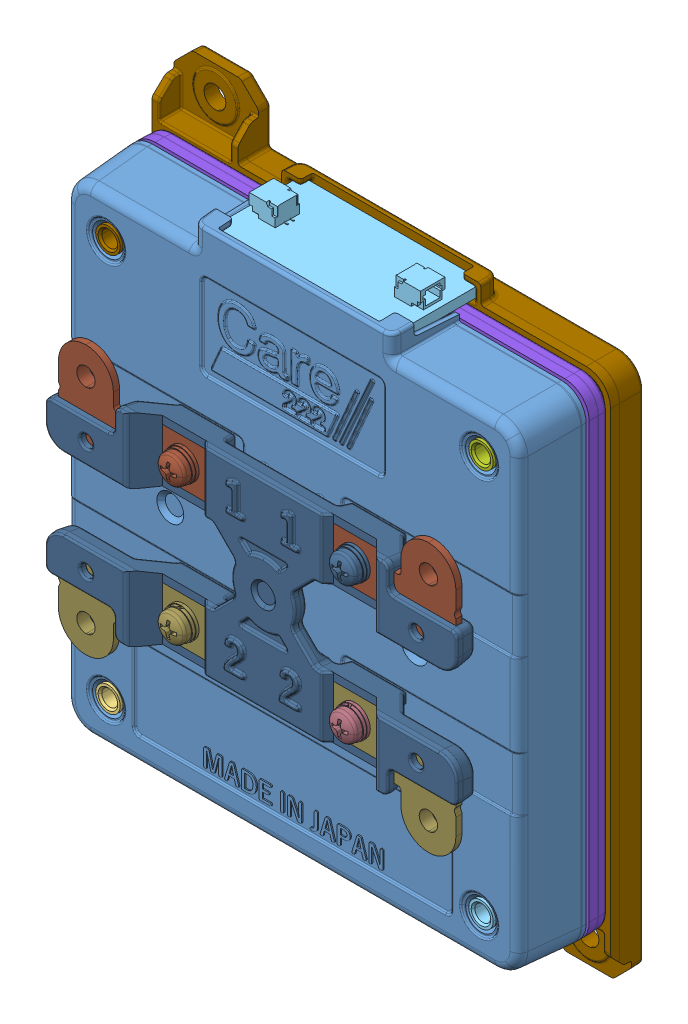
SolidWorks assembly emitter, configuration Default. Lengths in mm.
Overall size (75 97 26.91).
35 component instances, 31 part files, 0 mates.
Components (placement in the parent):
- emitter.step-1: emitter.step [Default] at origin size (75 97 26.91)
  - DRW1103739_UXFL70-222B4-UIA-Z1.STEP.step-1: DRW1103739_UXFL70-222B4-UIA-Z1.STEP.step [Default] at (-18.8418 87.9656 71.8261) size (75 97 26.91)
    - Z01_DRW1103184_LampCaseA.STEP.step-1: Z01_DRW1103184_LampCaseA.STEP.step [Default] at (0 3.0667 9.49) x (1 0 0) z (0 -1 0) size (75 10.8 82.07)
      - Z01_DRW1103184_LampCaseA-Part-1.STEP.step-1: Z01_DRW1103184_LampCaseA-Part-1.STEP.step [Default] at origin size (75 10.8 82.07)
      - Z01_DRW1103184_LampCaseA-Part-2.STEP.step-1: Z01_DRW1103184_LampCaseA-Part-2.STEP.step [Default] at origin size (4.3 4 4.3)
      - Z01_DRW1103184_LampCaseA-Part-3.STEP.step-1: Z01_DRW1103184_LampCaseA-Part-3.STEP.step [Default] at origin size (4.3 4 4.3)
      - Z01_DRW1103184_LampCaseA-Part-4.STEP.step-1: Z01_DRW1103184_LampCaseA-Part-4.STEP.step [Default] at origin size (4.3 4 4.3)
      - Z01_DRW1103184_LampCaseA-Part-5.STEP.step-1: Z01_DRW1103184_LampCaseA-Part-5.STEP.step [Default] at origin size (4.3 4 4.3)
      - Z01_DRW1103184_LampCaseA-Part-6.STEP.step-1: Z01_DRW1103184_LampCaseA-Part-6.STEP.step [Default] at origin size (4.3 4 4.3)
      - Z01_DRW1103184_LampCaseA-Part-7.STEP.step-1: Z01_DRW1103184_LampCaseA-Part-7.STEP.step [Default] at origin size (4.3 4 4.3)
      - Z01_DRW1103184_LampCaseA-Part-8.STEP.step-1: Z01_DRW1103184_LampCaseA-Part-8.STEP.step [Default] at origin size (4.3 4 4.3)
      - Z01_DRW1103184_LampCaseA-Part-9.STEP.step-1: Z01_DRW1103184_LampCaseA-Part-9.STEP.step [Default] at origin size (4.3 4 4.3)
    - Z14__[_q__X.STEP.step-1: Z14__[_q__X.STEP.step [Default] at (3.6282 -61.45 19.8) size (67.45 43.9 7.01)
      - Z14__[_q__X-Part-1.STEP.step-1: Z14__[_q__X-Part-1.STEP.step [Default] at origin size (67.45 33.11 7.01)
      - Z14__[_q__X-Part-2.STEP.step-1: Z14__[_q__X-Part-2.STEP.step [Default] at origin size (65 14.5 3)
      - Z14__[_q__X-Part-3.STEP.step-1: Z14__[_q__X-Part-3.STEP.step [Default] at origin size (65 14.5 3)
    - Z07_DRW1100980-01______70_~52.STEP.step-1: Z07_DRW1100980-01______70_~52.STEP.step [Default] at (4.525 -65.5 1.8) x (1 0 0) z (0 0 1) size (70 52 0.5)
    - Z10_222nm____.STEP.step-1: Z10_222nm____.STEP.step [Default] at (58.5 -67.1323 10) x (0 1 0) z (0 0 -1) size (68 6 6)
    - Z10_222nm____-1.STEP.step-1: Z10_222nm____-1.STEP.step [Default] at (44.5 -67.1323 10) x (0 1 0) z (0 0 -1) size (68 6 6)
    - Z10_222nm____-2.STEP.step-1: Z10_222nm____-2.STEP.step [Default] at (30.5 -67.1323 10) x (0 1 0) z (0 0 -1) size (68 6 6)
    - Z10_222nm____-3.STEP.step-1: Z10_222nm____-3.STEP.step [Default] at (16.5 -67.1323 10) x (0 1 0) z (0 0 -1) size (68 6 6)
    - Z11_222nmUV-BP____i.STEP.step-1: Z11_222nmUV-BP____i.STEP.step [Default] at (70.5 -13.5 2.3) x (-1 0 0) z (0 0 1) size (70 52 1)
    - Z08_W___(P4___a)__________M2.6_~12.STEP.step-1: Z08_W___(P4___a)__________M2.6_~12.STEP.step [Default] at (7 -72 0.8139) x (0 0 1) z (0 -1 0) size (13.67 5 5)
    - Z08_W___(P4___a)__________M2.6_~12-1.STEP.step-1: Z08_W___(P4___a)__________M2.6_~12-1.STEP.step [Default] at (68 -72 0.8139) x (0 0 1) z (0 -1 0) size (13.67 5 5)
    - Z08_W___(P4___a)__________M2.6_~12-2.STEP.step-1: Z08_W___(P4___a)__________M2.6_~12-2.STEP.step [Default] at (68 -7 0.8139) x (0 0 1) z (0 -1 0) size (13.67 5 5)
    - Z08_W___(P4___a)__________M2.6_~12-3.STEP.step-1: Z08_W___(P4___a)__________M2.6_~12-3.STEP.step [Default] at (7 -7 0.8139) x (0 0 1) z (0 -1 0) size (13.67 5 5)
    - Z12_LED____.STEP.step-1: Z12_LED____.STEP.step [Default] at (22.4997 -0.9256 18.6001) x (1 0 0.000001) z (0 1 0) size (30 15 5.81)
    - Z07_DRW1100980-01______70_~52-1.STEP.step-1: Z07_DRW1100980-01______70_~52-1.STEP.step [Default] at (4.525 -65.5 3.3) x (1 0 0) z (0 0 1) size (70 52 0.5)
    - Z13_LED_____h_~__.STEP.step-1: Z13_LED_____h_~__.STEP.step [Default] at (41.5 -2.15 10.5) x (0 0 1) z (0 -1 0) size (8 8 1)
    - Z02_DRW1103185_LampCaseB.STEP.step-1: Z02_DRW1103185_LampCaseB.STEP.step [Default] at (-151.9677 -5.0437 3.4157) size (75 79 12.5)
    - Z03_DRW1103186_LampCaseC.STEP.step-1: Z03_DRW1103186_LampCaseC.STEP.step [Default] at (0 -88 0) size (75 97 6.11)
    - Z08_W___(P4___a)__________M2.6_~12-4.STEP.step-1: Z08_W___(P4___a)__________M2.6_~12-4.STEP.step [Default] at (51.5 -28.3 26.4861) x (0 0 -1) z (0 -1 0) size (13.67 5 5)
    - Z08_W___(P4___a)__________M2.6_~12-5.STEP.step-1: Z08_W___(P4___a)__________M2.6_~12-5.STEP.step [Default] at (23.5 -28.3 26.4861) x (0 0 -1) z (0 -1 0) size (13.67 5 5)
    - Z08_W___(P4___a)__________M2.6_~12-6.STEP.step-1: Z08_W___(P4___a)__________M2.6_~12-6.STEP.step [Default] at (23.5 -50.7 26.4861) x (0 0 -1) z (0 1 0) size (13.67 5 5)
    - Z08_W___(P4___a)__________M2.6_~12-7.STEP.step-1: Z08_W___(P4___a)__________M2.6_~12-7.STEP.step [Default] at (51.5 -50.7 26.4861) x (0 0 -1) z (0 1 0) size (13.67 5 5)
